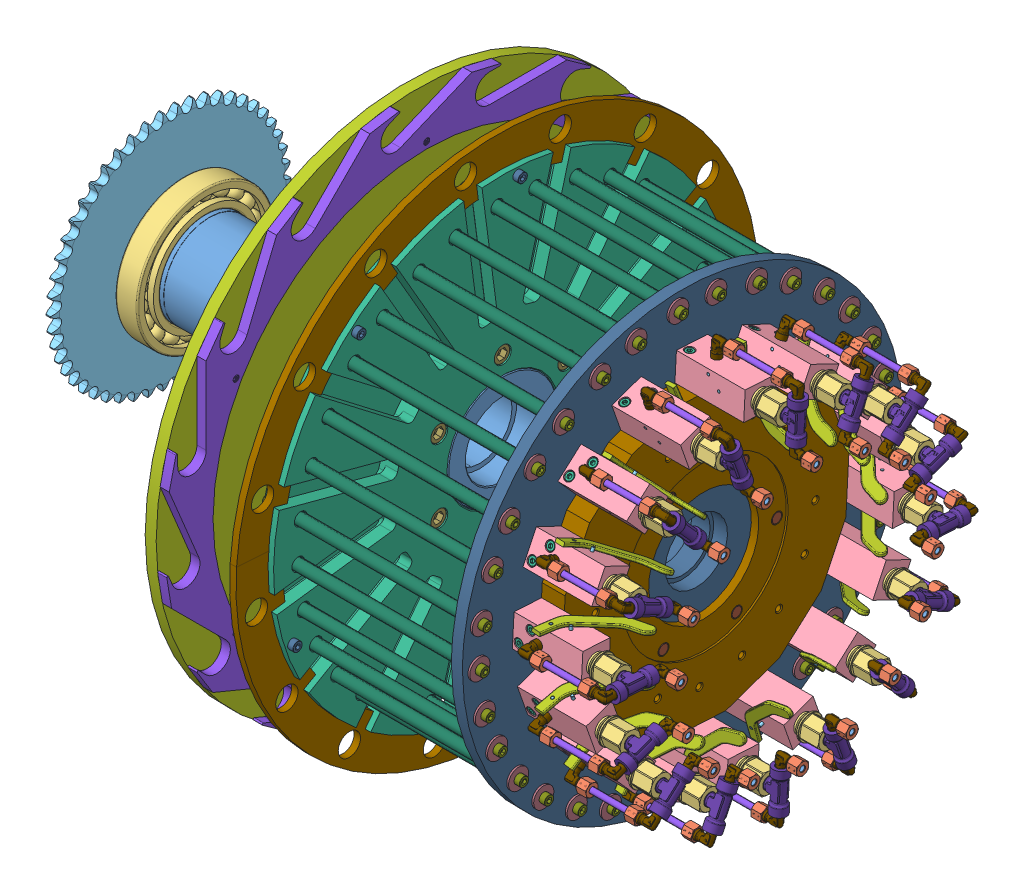
SolidWorks assembly assieme parte rotante, configuration Default. Lengths in mm.
Overall size (749.63 778.63 778.63).
555 component instances, 28 part files, 77 mates.
Components (placement in the parent):
- albero rotazione piatti-1: albero rotazione piatti [Default] at (60.413 18.3637 415) size (415 200 200)
- seger 100mm-1: seger 100mm [KS 1336 E - 100] at (-146.4567 18.3637 415) x (0 0 -1) z (1 0 0) size (107.55 112.98 3)
- SKF - 6020 - 20,DE,NC,20_68-1: SKF - 6020 - 20,DE,NC,20_68 [SKF - 6020 - 20,DE,NC,20_68] at (-131.4567 18.3637 415) x (1 0 0) z (0 -0.434476 -0.900684) size (24 150 150)
- calettatore d95-1: calettatore d95 [Default] at (-178.8867 18.3637 415) size (39.5 135 135)
- Chain wheel ISO - 50Z 10A-1-1: Chain wheel ISO - 50Z 10A-1 [Chain wheel ISO - 50Z 10A-1 --50SB120H25L95.0N] at (-164.8867 18.3637 415) size (33.93 262.06 262.51)
- Disco supporto montaggio e Colonne-1: Disco supporto montaggio e Colonne [Default] at (204.0433 18.3637 415) x (0 -0.866025 -0.5) z (1 0 0) size (499.6 499.6 29)
- SKF - 6020 - 20,DE,NC,20_68-2: SKF - 6020 - 20,DE,NC,20_68 [SKF - 6020 - 20,DE,NC,20_68] at (62.0433 18.3637 415) x (1 0 0) z (0 -0.432628 -0.901573) size (24 150 150)
- piatto rotante porta tappi-1: piatto rotante porta tappi [Default] at (99.0433 18.3637 415) x (0 0 -1) z (1 0 0) size (570 570 20.57)
- disco trasportatore tappi 31-1: disco trasportatore tappi 31 [Default] at (111.0433 18.3637 415) x (0 0.5 -0.866025) z (1 0 0) size (570 570 10.42)
- Distributore Rotante-1: Distributore Rotante [Default] at (425.0433 18.3637 415) x (0 -0.055301 -0.99847) z (1 0 0) size (310 310 25.54)
- disco trascinato porta distributore vuoto-1: disco trascinato porta distributore vuoto [Default] at (400.0433 18.3637 415) x (0 0.055301 0.99847) z (-1 0 0) size (480 480 50)
- m12 35mm-1: m12 35mm [ISO 4762 M12 x 35 - 35N] at (376.0433 -53.0243 378.8925) x (1 0 0) z (0 -0.5 0.866025) size (47 18 18)
- m12 90mm-3: m12 90mm [ISO 4762 M12 x 90 - 90N] at (203.0433 -21.6363 345.718) x (-1 0 0) z (0 -0.5 0.866025) size (102 18 18)
- rondella m6 22mm-1: rondella m6 22mm [Washer ISO 7094 - 6] at (99.0433 -101.6363 207.1539) x (1 0 0) z (0 -1 0) size (2 22 22)
- M6 20mm-1: M6 20mm [ISO 4762 M6 x 20 - 20N] at (91.0433 -101.6363 207.1539) x (1 0 0) z (0 0.5 0.866025) size (26 10 10)
- m12 35mm-2: m12 35mm [ISO 4762 M12 x 35 - 35N] at (376.0433 13.9397 335.1224) x (1 0 0) z (0 -1 0) size (47 18 18)
- m12 35mm-3: m12 35mm [ISO 4762 M12 x 35 - 35N] at (376.0433 85.3277 371.2299) x (1 0 0) z (0 -0.5 -0.866025) size (47 18 18)
- m12 35mm-4: m12 35mm [ISO 4762 M12 x 35 - 35N] at (376.0433 89.7517 451.1075) x (1 0 0) z (0 0.5 -0.866025) size (47 18 18)
- m12 35mm-5: m12 35mm [ISO 4762 M12 x 35 - 35N] at (376.0433 22.7877 494.8776) x (1 0 0) z (0 1 0) size (47 18 18)
- m12 35mm-6: m12 35mm [ISO 4762 M12 x 35 - 35N] at (376.0433 -48.6003 458.7701) x (1 0 0) z (0 0.5 0.866025) size (47 18 18)
- rondella m6 22mm-2: rondella m6 22mm [Washer ISO 7094 - 6] at (99.0433 138.3637 207.1539) x (1 0 0) z (0 -0.5 -0.866025) size (2 22 22)
- rondella m6 22mm-3: rondella m6 22mm [Washer ISO 7094 - 6] at (99.0433 258.3637 415) x (1 0 0) z (0 0.5 -0.866025) size (2 22 22)
- rondella m6 22mm-4: rondella m6 22mm [Washer ISO 7094 - 6] at (99.0433 138.3637 622.8461) x (1 0 0) z (0 1 0) size (2 22 22)
- rondella m6 22mm-5: rondella m6 22mm [Washer ISO 7094 - 6] at (99.0433 -101.6363 622.8461) x (1 0 0) z (0 0.5 0.866025) size (2 22 22)
- rondella m6 22mm-6: rondella m6 22mm [Washer ISO 7094 - 6] at (99.0433 -221.6363 415) x (1 0 0) z (0 -0.5 0.866025) size (2 22 22)
- M6 20mm-2: M6 20mm [ISO 4762 M6 x 20 - 20N] at (91.0433 138.3637 207.1539) x (1 0 0) z (0 -0.5 0.866025) size (26 10 10)
- M6 20mm-3: M6 20mm [ISO 4762 M6 x 20 - 20N] at (91.0433 258.3637 415) x (1 0 0) z (0 -1 0) size (26 10 10)
- M6 20mm-4: M6 20mm [ISO 4762 M6 x 20 - 20N] at (91.0433 138.3637 622.8461) x (1 0 0) z (0 -0.5 -0.866025) size (26 10 10)
- M6 20mm-5: M6 20mm [ISO 4762 M6 x 20 - 20N] at (91.0433 -101.6363 622.8461) x (1 0 0) z (0 0.5 -0.866025) size (26 10 10)
- M6 20mm-6: M6 20mm [ISO 4762 M6 x 20 - 20N] at (91.0433 -221.6363 415) x (1 0 0) z (0 1 0) size (26 10 10)
- m12 90mm-4: m12 90mm [ISO 4762 M12 x 90 - 90N] at (203.0433 58.3637 345.718) x (-1 0 0) z (0 -1 0) size (102 18 18)
- m12 90mm-5: m12 90mm [ISO 4762 M12 x 90 - 90N] at (203.0433 98.3637 415) x (-1 0 0) z (0 -0.5 -0.866025) size (102 18 18)
- m12 90mm-6: m12 90mm [ISO 4762 M12 x 90 - 90N] at (203.0433 58.3637 484.282) x (-1 0 0) z (0 0.5 -0.866025) size (102 18 18)
- m12 90mm-7: m12 90mm [ISO 4762 M12 x 90 - 90N] at (203.0433 -21.6363 484.282) x (-1 0 0) z (0 1 0) size (102 18 18)
- m12 90mm-8: m12 90mm [ISO 4762 M12 x 90 - 90N] at (203.0433 -61.6363 415) x (-1 0 0) z (0 0.5 0.866025) size (102 18 18)
- asta scorrimento carello-1: asta scorrimento carello [Default] at (287.5433 70.1437 197.9013) x (0 0 -1) z (1 0 0) size (12 12 225)
- rondella m6 22mm-7: rondella m6 22mm [Washer ISO 7094 - 6] at (175.0433 70.1437 197.9013) x (1 0 0) z (0 -1 0) size (2 22 22)
- M6 16mm-1: M6 16mm [ISO 4762 M6 x 16 - 16N] at (167.0433 70.1437 197.9013) size (22 10 10)
- M6 16mm-2: M6 16mm [ISO 4762 M6 x 16 - 16N] at (408.0433 70.1437 197.9013) x (-1 0 0) z (0 0 -1) size (22 10 10)
- rondella m6 22mm-8: rondella m6 22mm [Washer ISO 7094 - 6] at (400.0433 70.1437 197.9013) x (-1 0 0) z (0 1 0) size (2 22 22)
- rondella m6 22mm-9: rondella m6 22mm [Washer ISO 7094 - 6] at (175.0433 24.5373 191.8971) x (1 0 0) z (0 -0.965926 -0.258819) size (2 22 22)
- M6 16mm-3: M6 16mm [ISO 4762 M6 x 16 - 16N] at (167.0433 24.5373 191.8971) x (1 0 0) z (0 0.258819 -0.965926) size (22 10 10)
- asta scorrimento carello-2: asta scorrimento carello [Default] at (287.5433 24.5373 191.8971) x (0 0.258819 -0.965926) z (-1 0 0) size (12 12 225)
- rondella m6 22mm-10: rondella m6 22mm [Washer ISO 7094 - 6] at (400.0433 24.5373 191.8971) x (-1 0 0) z (0 0.965926 0.258819) size (2 22 22)
- M6 16mm-4: M6 16mm [ISO 4762 M6 x 16 - 16N] at (408.0433 24.5373 191.8971) x (-1 0 0) z (0 -0.258819 0.965926) size (22 10 10)
- AssiemeValvola-1: AssiemeValvola [Default] at (515.3257 74.6348 254.5832) x (0 -0.331007 0.943628) z (0 0.943628 0.331007) size (90.26 138.63 38)
  - RaccordoT-1: RaccordoT [Default] at origin size (43 29.75 16.5)
  - Raccordo a L-1: Raccordo a L [Default] at (-30 0 0) x (0 -1 0) z (0 0 -1) size (28.34 25.51 14.01)
    - 1809_06_10_01-1: 1809_06_10_01 [Default] at origin size (22.49 23 10)
    - 1809_06_10_02-1: 1809_06_10_02 [Default] at origin size (6.5 8.5 8.5)
    - 1809_06_10_03-1: 1809_06_10_03 [Default] at origin size (11.02 15.01 14.01)
  - Raccordo a L-2: Raccordo a L [Default] at (30 0 0) x (0 1 0) z (0 0 -1) size (28.34 25.51 14.01)
    - 1809_06_10_01-1: 1809_06_10_01 [Default] at origin size (22.49 23 10)
    - 1809_06_10_02-1: 1809_06_10_02 [Default] at origin size (6.5 8.5 8.5)
    - 1809_06_10_03-1: 1809_06_10_03 [Default] at origin size (11.02 15.01 14.01)
  - TappoChiusura-1: TappoChiusura [Default] at (0 -32 0) x (0 -1 0) z (0 0 1) size (38.28 26.74 26.74)
  - CorpoValvola-1: CorpoValvola [Default] at (-15 -115.2824 0) size (30 75 34)
  - Raccordo a L-3: Raccordo a L [Default] at (-30 -88.2824 0) x (0 1 0) z (0 0 1) size (28.34 25.51 14.01)
    - 1809_06_10_01-1: 1809_06_10_01 [Default] at origin size (22.49 23 10)
    - 1809_06_10_02-1: 1809_06_10_02 [Default] at origin size (6.5 8.5 8.5)
    - 1809_06_10_03-1: 1809_06_10_03 [Default] at origin size (11.02 15.01 14.01)
  - Spina_3x38-1: Spina_3x38 [Default] at (0 -68.2824 -21) x (-1 0 0) z (0 0 1) size (3 3 38)
  - Spina_3x38-2: Spina_3x38 [Default] at (-10 -80.2824 -21) x (0.996193 0.087174 0) z (0 0 1) size (3 3 38)
  - M5 40mm-3: M5 40mm [ISO 4762 M5 x 40 - 40N] at (-14.6 -108.7824 9) size (45 8.5 8.5)
  - M5 40mm-2: M5 40mm [ISO 4762 M5 x 40 - 40N] at (-14.6 -96.7824 -9) size (45 8.5 8.5)
  - LevaValvola-1: LevaValvola [Default] at (-24.507 -86.571 -17) x (0.996193 0.087174 0) z (0 0 1) size (77.55 60.2 4)
  - Tubo-1: Tubo [Default] at (-30 -15.9665 0) x (1 0 0) z (0 -1 0) size (6 6 56.4)
- M6 16mm-5: M6 16mm [ISO 4762 M6 x 16 - 16N] at (167.0433 -16.8778 194.6116) x (1 0 0) z (0 0.382683 0.92388) size (22 10 10)
- M6 16mm-6: M6 16mm [ISO 4762 M6 x 16 - 16N] at (167.0433 -98.5342 224.874) x (1 0 0) z (0 0.707107 0.707107) size (22 10 10)
- M6 16mm-7: M6 16mm [ISO 4762 M6 x 16 - 16N] at (167.0433 -162.3939 284.0814) x (1 0 0) z (0 0.92388 0.382683) size (22 10 10)
- M6 16mm-8: M6 16mm [ISO 4762 M6 x 16 - 16N] at (167.0433 -198.735 363.22) x (1 0 0) z (0 1 0) size (22 10 10)
- M6 16mm-9: M6 16mm [ISO 4762 M6 x 16 - 16N] at (167.0433 -202.0247 450.2415) x (1 0 0) z (0 0.92388 -0.382683) size (22 10 10)
- M6 16mm-10: M6 16mm [ISO 4762 M6 x 16 - 16N] at (167.0433 -171.7623 531.8979) x (1 0 0) z (0 0.707107 -0.707107) size (22 10 10)
- M6 16mm-11: M6 16mm [ISO 4762 M6 x 16 - 16N] at (167.0433 -112.5549 595.7576) x (1 0 0) z (0 0.382683 -0.92388) size (22 10 10)
- M6 16mm-12: M6 16mm [ISO 4762 M6 x 16 - 16N] at (167.0433 -33.4163 632.0987) x (1 0 0) z (0 0 -1) size (22 10 10)
- M6 16mm-13: M6 16mm [ISO 4762 M6 x 16 - 16N] at (167.0433 53.6052 635.3884) x (1 0 0) z (0 -0.382683 -0.92388) size (22 10 10)
- M6 16mm-14: M6 16mm [ISO 4762 M6 x 16 - 16N] at (167.0433 135.2616 605.126) x (1 0 0) z (0 -0.707107 -0.707107) size (22 10 10)
- M6 16mm-15: M6 16mm [ISO 4762 M6 x 16 - 16N] at (167.0433 199.1213 545.9186) x (1 0 0) z (0 -0.92388 -0.382683) size (22 10 10)
- M6 16mm-16: M6 16mm [ISO 4762 M6 x 16 - 16N] at (167.0433 235.4624 466.78) x (1 0 0) z (0 -1 0) size (22 10 10)
- M6 16mm-17: M6 16mm [ISO 4762 M6 x 16 - 16N] at (167.0433 238.7521 379.7585) x (1 0 0) z (0 -0.92388 0.382683) size (22 10 10)
- M6 16mm-18: M6 16mm [ISO 4762 M6 x 16 - 16N] at (167.0433 208.4897 298.1021) x (1 0 0) z (0 -0.707107 0.707107) size (22 10 10)
- M6 16mm-19: M6 16mm [ISO 4762 M6 x 16 - 16N] at (167.0433 149.2823 234.2424) x (1 0 0) z (0 -0.382683 0.92388) size (22 10 10)
- rondella m6 22mm-11: rondella m6 22mm [Washer ISO 7094 - 6] at (175.0433 -16.8778 194.6116) x (1 0 0) z (0 -0.92388 0.382683) size (2 22 22)
- rondella m6 22mm-12: rondella m6 22mm [Washer ISO 7094 - 6] at (175.0433 -98.5342 224.874) x (1 0 0) z (0 -0.707107 0.707107) size (2 22 22)
- rondella m6 22mm-13: rondella m6 22mm [Washer ISO 7094 - 6] at (175.0433 -162.3939 284.0814) x (1 0 0) z (0 -0.382683 0.92388) size (2 22 22)
- rondella m6 22mm-14: rondella m6 22mm [Washer ISO 7094 - 6] at (175.0433 -198.735 363.22) size (2 22 22)
- rondella m6 22mm-15: rondella m6 22mm [Washer ISO 7094 - 6] at (175.0433 -202.0247 450.2415) x (1 0 0) z (0 0.382683 0.92388) size (2 22 22)
- rondella m6 22mm-16: rondella m6 22mm [Washer ISO 7094 - 6] at (175.0433 -171.7623 531.8979) x (1 0 0) z (0 0.707107 0.707107) size (2 22 22)
- rondella m6 22mm-17: rondella m6 22mm [Washer ISO 7094 - 6] at (175.0433 -112.5549 595.7576) x (1 0 0) z (0 0.92388 0.382683) size (2 22 22)
- rondella m6 22mm-18: rondella m6 22mm [Washer ISO 7094 - 6] at (175.0433 -33.4163 632.0987) x (1 0 0) z (0 1 0) size (2 22 22)
- rondella m6 22mm-19: rondella m6 22mm [Washer ISO 7094 - 6] at (175.0433 53.6052 635.3884) x (1 0 0) z (0 0.92388 -0.382683) size (2 22 22)
- rondella m6 22mm-20: rondella m6 22mm [Washer ISO 7094 - 6] at (175.0433 135.2616 605.126) x (1 0 0) z (0 0.707107 -0.707107) size (2 22 22)
- rondella m6 22mm-21: rondella m6 22mm [Washer ISO 7094 - 6] at (175.0433 199.1213 545.9186) x (1 0 0) z (0 0.382683 -0.92388) size (2 22 22)
- rondella m6 22mm-22: rondella m6 22mm [Washer ISO 7094 - 6] at (175.0433 235.4624 466.78) x (1 0 0) z (0 0 -1) size (2 22 22)
- rondella m6 22mm-23: rondella m6 22mm [Washer ISO 7094 - 6] at (175.0433 238.7521 379.7585) x (1 0 0) z (0 -0.382683 -0.92388) size (2 22 22)
- rondella m6 22mm-24: rondella m6 22mm [Washer ISO 7094 - 6] at (175.0433 208.4897 298.1021) x (1 0 0) z (0 -0.707107 -0.707107) size (2 22 22)
- rondella m6 22mm-25: rondella m6 22mm [Washer ISO 7094 - 6] at (175.0433 149.2823 234.2424) x (1 0 0) z (0 -0.92388 -0.382683) size (2 22 22)
- asta scorrimento carello-3: asta scorrimento carello [Default] at (287.5433 -16.8778 194.6116) x (0 -0.382683 -0.92388) z (1 0 0) size (12 12 225)
- asta scorrimento carello-4: asta scorrimento carello [Default] at (287.5433 -98.5342 224.874) x (0 -0.707107 -0.707107) z (1 0 0) size (12 12 225)
- asta scorrimento carello-5: asta scorrimento carello [Default] at (287.5433 -162.3939 284.0814) x (0 -0.92388 -0.382683) z (1 0 0) size (12 12 225)
- asta scorrimento carello-6: asta scorrimento carello [Default] at (287.5433 -198.735 363.22) x (0 -1 0) z (1 0 0) size (12 12 225)
- asta scorrimento carello-7: asta scorrimento carello [Default] at (287.5433 -202.0247 450.2415) x (0 -0.92388 0.382683) z (1 0 0) size (12 12 225)
- asta scorrimento carello-8: asta scorrimento carello [Default] at (287.5433 -171.7623 531.8979) x (0 -0.707107 0.707107) z (1 0 0) size (12 12 225)
- asta scorrimento carello-9: asta scorrimento carello [Default] at (287.5433 -112.5549 595.7576) x (0 -0.382683 0.92388) z (1 0 0) size (12 12 225)
- asta scorrimento carello-10: asta scorrimento carello [Default] at (287.5433 -33.4163 632.0987) x (0 0 1) z (1 0 0) size (12 12 225)
- asta scorrimento carello-11: asta scorrimento carello [Default] at (287.5433 53.6052 635.3884) x (0 0.382683 0.92388) z (1 0 0) size (12 12 225)
- asta scorrimento carello-12: asta scorrimento carello [Default] at (287.5433 135.2616 605.126) x (0 0.707107 0.707107) z (1 0 0) size (12 12 225)
- asta scorrimento carello-13: asta scorrimento carello [Default] at (287.5433 199.1213 545.9186) x (0 0.92388 0.382683) z (1 0 0) size (12 12 225)
- asta scorrimento carello-14: asta scorrimento carello [Default] at (287.5433 235.4624 466.78) x (0 1 0) z (1 0 0) size (12 12 225)
- asta scorrimento carello-15: asta scorrimento carello [Default] at (287.5433 238.7521 379.7585) x (0 0.92388 -0.382683) z (1 0 0) size (12 12 225)
- asta scorrimento carello-16: asta scorrimento carello [Default] at (287.5433 208.4897 298.1021) x (0 0.707107 -0.707107) z (1 0 0) size (12 12 225)
- asta scorrimento carello-17: asta scorrimento carello [Default] at (287.5433 149.2823 234.2424) x (0 0.382683 -0.92388) z (1 0 0) size (12 12 225)
- M6 16mm-20: M6 16mm [ISO 4762 M6 x 16 - 16N] at (408.0433 -16.8778 194.6116) x (-1 0 0) z (0 -0.382683 -0.92388) size (22 10 10)
- M6 16mm-21: M6 16mm [ISO 4762 M6 x 16 - 16N] at (408.0433 -98.5342 224.874) x (-1 0 0) z (0 -0.707107 -0.707107) size (22 10 10)
- M6 16mm-22: M6 16mm [ISO 4762 M6 x 16 - 16N] at (408.0433 -162.3939 284.0814) x (-1 0 0) z (0 -0.92388 -0.382683) size (22 10 10)
- M6 16mm-23: M6 16mm [ISO 4762 M6 x 16 - 16N] at (408.0433 -198.735 363.22) x (-1 0 0) z (0 -1 0) size (22 10 10)
- M6 16mm-24: M6 16mm [ISO 4762 M6 x 16 - 16N] at (408.0433 -202.0247 450.2415) x (-1 0 0) z (0 -0.92388 0.382683) size (22 10 10)
- M6 16mm-25: M6 16mm [ISO 4762 M6 x 16 - 16N] at (408.0433 -171.7623 531.8979) x (-1 0 0) z (0 -0.707107 0.707107) size (22 10 10)
- M6 16mm-26: M6 16mm [ISO 4762 M6 x 16 - 16N] at (408.0433 -112.5549 595.7576) x (-1 0 0) z (0 -0.382683 0.92388) size (22 10 10)
- M6 16mm-27: M6 16mm [ISO 4762 M6 x 16 - 16N] at (408.0433 -33.4163 632.0987) x (-1 0 0) z (0 0 1) size (22 10 10)
- M6 16mm-28: M6 16mm [ISO 4762 M6 x 16 - 16N] at (408.0433 53.6052 635.3884) x (-1 0 0) z (0 0.382683 0.92388) size (22 10 10)
- M6 16mm-29: M6 16mm [ISO 4762 M6 x 16 - 16N] at (408.0433 135.2616 605.126) x (-1 0 0) z (0 0.707107 0.707107) size (22 10 10)
- M6 16mm-30: M6 16mm [ISO 4762 M6 x 16 - 16N] at (408.0433 199.1213 545.9186) x (-1 0 0) z (0 0.92388 0.382683) size (22 10 10)
- M6 16mm-31: M6 16mm [ISO 4762 M6 x 16 - 16N] at (408.0433 235.4624 466.78) x (-1 0 0) z (0 1 0) size (22 10 10)
- M6 16mm-32: M6 16mm [ISO 4762 M6 x 16 - 16N] at (408.0433 238.7521 379.7585) x (-1 0 0) z (0 0.92388 -0.382683) size (22 10 10)
- M6 16mm-33: M6 16mm [ISO 4762 M6 x 16 - 16N] at (408.0433 208.4897 298.1021) x (-1 0 0) z (0 0.707107 -0.707107) size (22 10 10)
- M6 16mm-34: M6 16mm [ISO 4762 M6 x 16 - 16N] at (408.0433 149.2823 234.2424) x (-1 0 0) z (0 0.382683 -0.92388) size (22 10 10)
- rondella m6 22mm-26: rondella m6 22mm [Washer ISO 7094 - 6] at (400.0433 -16.8778 194.6116) x (-1 0 0) z (0 0.92388 -0.382683) size (2 22 22)
- rondella m6 22mm-27: rondella m6 22mm [Washer ISO 7094 - 6] at (400.0433 -98.5342 224.874) x (-1 0 0) z (0 0.707107 -0.707107) size (2 22 22)
- rondella m6 22mm-28: rondella m6 22mm [Washer ISO 7094 - 6] at (400.0433 -162.3939 284.0814) x (-1 0 0) z (0 0.382683 -0.92388) size (2 22 22)
- rondella m6 22mm-29: rondella m6 22mm [Washer ISO 7094 - 6] at (400.0433 -198.735 363.22) x (-1 0 0) z (0 0 -1) size (2 22 22)
- rondella m6 22mm-30: rondella m6 22mm [Washer ISO 7094 - 6] at (400.0433 -202.0247 450.2415) x (-1 0 0) z (0 -0.382683 -0.92388) size (2 22 22)
- rondella m6 22mm-31: rondella m6 22mm [Washer ISO 7094 - 6] at (400.0433 -171.7623 531.8979) x (-1 0 0) z (0 -0.707107 -0.707107) size (2 22 22)
- rondella m6 22mm-32: rondella m6 22mm [Washer ISO 7094 - 6] at (400.0433 -112.5549 595.7576) x (-1 0 0) z (0 -0.92388 -0.382683) size (2 22 22)
- rondella m6 22mm-33: rondella m6 22mm [Washer ISO 7094 - 6] at (400.0433 -33.4163 632.0987) x (-1 0 0) z (0 -1 0) size (2 22 22)
- rondella m6 22mm-34: rondella m6 22mm [Washer ISO 7094 - 6] at (400.0433 53.6052 635.3884) x (-1 0 0) z (0 -0.92388 0.382683) size (2 22 22)
- rondella m6 22mm-35: rondella m6 22mm [Washer ISO 7094 - 6] at (400.0433 135.2616 605.126) x (-1 0 0) z (0 -0.707107 0.707107) size (2 22 22)
- rondella m6 22mm-36: rondella m6 22mm [Washer ISO 7094 - 6] at (400.0433 199.1213 545.9186) x (-1 0 0) z (0 -0.382683 0.92388) size (2 22 22)
- rondella m6 22mm-37: rondella m6 22mm [Washer ISO 7094 - 6] at (400.0433 235.4624 466.78) x (-1 0 0) z (0 0 1) size (2 22 22)
- rondella m6 22mm-38: rondella m6 22mm [Washer ISO 7094 - 6] at (400.0433 238.7521 379.7585) x (-1 0 0) z (0 0.382683 0.92388) size (2 22 22)
- rondella m6 22mm-39: rondella m6 22mm [Washer ISO 7094 - 6] at (400.0433 208.4897 298.1021) x (-1 0 0) z (0 0.707107 0.707107) size (2 22 22)
- rondella m6 22mm-40: rondella m6 22mm [Washer ISO 7094 - 6] at (400.0433 149.2823 234.2424) x (-1 0 0) z (0 0.92388 0.382683) size (2 22 22)
- rondella m6 22mm-41: rondella m6 22mm [Washer ISO 7094 - 6] at (175.0433 -61.3104 206.5173) x (1 0 0) z (0 -0.991445 0.130526) size (2 22 22)
- rondella m6 22mm-42: rondella m6 22mm [Washer ISO 7094 - 6] at (175.0433 -135.0285 252.8771) x (1 0 0) z (0 -0.866025 0.5) size (2 22 22)
- rondella m6 22mm-43: rondella m6 22mm [Washer ISO 7094 - 6] at (175.0433 -185.3939 323.9186) x (1 0 0) z (0 -0.608761 0.793353) size (2 22 22)
- rondella m6 22mm-44: rondella m6 22mm [Washer ISO 7094 - 6] at (175.0433 -204.7392 408.8264) x (1 0 0) z (0 -0.258819 0.965926) size (2 22 22)
- rondella m6 22mm-45: rondella m6 22mm [Washer ISO 7094 - 6] at (175.0433 -190.119 494.6741) x (1 0 0) z (0 0.130526 0.991445) size (2 22 22)
- rondella m6 22mm-46: rondella m6 22mm [Washer ISO 7094 - 6] at (175.0433 -143.7592 568.3922) x (1 0 0) z (0 0.5 0.866025) size (2 22 22)
- rondella m6 22mm-47: rondella m6 22mm [Washer ISO 7094 - 6] at (175.0433 -72.7177 618.7576) x (1 0 0) z (0 0.793353 0.608761) size (2 22 22)
- rondella m6 22mm-48: rondella m6 22mm [Washer ISO 7094 - 6] at (175.0433 12.1901 638.1029) x (1 0 0) z (0 0.965926 0.258819) size (2 22 22)
- rondella m6 22mm-49: rondella m6 22mm [Washer ISO 7094 - 6] at (175.0433 98.0378 623.4827) x (1 0 0) z (0 0.991445 -0.130526) size (2 22 22)
- rondella m6 22mm-50: rondella m6 22mm [Washer ISO 7094 - 6] at (175.0433 171.7559 577.1229) x (1 0 0) z (0 0.866025 -0.5) size (2 22 22)
- rondella m6 22mm-51: rondella m6 22mm [Washer ISO 7094 - 6] at (175.0433 222.1213 506.0814) x (1 0 0) z (0 0.608761 -0.793353) size (2 22 22)
- rondella m6 22mm-52: rondella m6 22mm [Washer ISO 7094 - 6] at (175.0433 241.4666 421.1736) x (1 0 0) z (0 0.258819 -0.965926) size (2 22 22)
- rondella m6 22mm-53: rondella m6 22mm [Washer ISO 7094 - 6] at (175.0433 226.8464 335.3259) x (1 0 0) z (0 -0.130526 -0.991445) size (2 22 22)
- rondella m6 22mm-54: rondella m6 22mm [Washer ISO 7094 - 6] at (175.0433 180.4866 261.6078) x (1 0 0) z (0 -0.5 -0.866025) size (2 22 22)
- rondella m6 22mm-55: rondella m6 22mm [Washer ISO 7094 - 6] at (175.0433 109.4451 211.2424) x (1 0 0) z (0 -0.793353 -0.608761) size (2 22 22)
- M6 16mm-35: M6 16mm [ISO 4762 M6 x 16 - 16N] at (167.0433 -61.3104 206.5173) x (1 0 0) z (0 -0.130526 -0.991445) size (22 10 10)
- M6 16mm-36: M6 16mm [ISO 4762 M6 x 16 - 16N] at (167.0433 -135.0285 252.8771) x (1 0 0) z (0 -0.5 -0.866025) size (22 10 10)
- M6 16mm-37: M6 16mm [ISO 4762 M6 x 16 - 16N] at (167.0433 -185.3939 323.9186) x (1 0 0) z (0 -0.793353 -0.608761) size (22 10 10)
- M6 16mm-38: M6 16mm [ISO 4762 M6 x 16 - 16N] at (167.0433 -204.7392 408.8264) x (1 0 0) z (0 -0.965926 -0.258819) size (22 10 10)
- M6 16mm-39: M6 16mm [ISO 4762 M6 x 16 - 16N] at (167.0433 -190.119 494.6741) x (1 0 0) z (0 -0.991445 0.130526) size (22 10 10)
- M6 16mm-40: M6 16mm [ISO 4762 M6 x 16 - 16N] at (167.0433 -143.7592 568.3922) x (1 0 0) z (0 -0.866025 0.5) size (22 10 10)
- M6 16mm-41: M6 16mm [ISO 4762 M6 x 16 - 16N] at (167.0433 -72.7177 618.7576) x (1 0 0) z (0 -0.608761 0.793353) size (22 10 10)
- M6 16mm-42: M6 16mm [ISO 4762 M6 x 16 - 16N] at (167.0433 12.1901 638.1029) x (1 0 0) z (0 -0.258819 0.965926) size (22 10 10)
- M6 16mm-43: M6 16mm [ISO 4762 M6 x 16 - 16N] at (167.0433 98.0378 623.4827) x (1 0 0) z (0 0.130526 0.991445) size (22 10 10)
- M6 16mm-44: M6 16mm [ISO 4762 M6 x 16 - 16N] at (167.0433 171.7559 577.1229) x (1 0 0) z (0 0.5 0.866025) size (22 10 10)
- M6 16mm-45: M6 16mm [ISO 4762 M6 x 16 - 16N] at (167.0433 222.1213 506.0814) x (1 0 0) z (0 0.793353 0.608761) size (22 10 10)
- M6 16mm-46: M6 16mm [ISO 4762 M6 x 16 - 16N] at (167.0433 241.4666 421.1736) x (1 0 0) z (0 0.965926 0.258819) size (22 10 10)
- M6 16mm-47: M6 16mm [ISO 4762 M6 x 16 - 16N] at (167.0433 226.8464 335.3259) x (1 0 0) z (0 0.991445 -0.130526) size (22 10 10)
- M6 16mm-48: M6 16mm [ISO 4762 M6 x 16 - 16N] at (167.0433 180.4866 261.6078) x (1 0 0) z (0 0.866025 -0.5) size (22 10 10)
- M6 16mm-49: M6 16mm [ISO 4762 M6 x 16 - 16N] at (167.0433 109.4451 211.2424) x (1 0 0) z (0 0.608761 -0.793353) size (22 10 10)
- asta scorrimento carello-18: asta scorrimento carello [Default] at (287.5433 -61.3104 206.5173) x (0 -0.130526 -0.991445) z (-1 0 0) size (12 12 225)
- asta scorrimento carello-19: asta scorrimento carello [Default] at (287.5433 -135.0285 252.8771) x (0 -0.5 -0.866025) z (-1 0 0) size (12 12 225)
- asta scorrimento carello-20: asta scorrimento carello [Default] at (287.5433 -185.3939 323.9186) x (0 -0.793353 -0.608761) z (-1 0 0) size (12 12 225)
- asta scorrimento carello-21: asta scorrimento carello [Default] at (287.5433 -204.7392 408.8264) x (0 -0.965926 -0.258819) z (-1 0 0) size (12 12 225)
- asta scorrimento carello-22: asta scorrimento carello [Default] at (287.5433 -190.119 494.6741) x (0 -0.991445 0.130526) z (-1 0 0) size (12 12 225)
- asta scorrimento carello-23: asta scorrimento carello [Default] at (287.5433 -143.7592 568.3922) x (0 -0.866025 0.5) z (-1 0 0) size (12 12 225)
- asta scorrimento carello-24: asta scorrimento carello [Default] at (287.5433 -72.7177 618.7576) x (0 -0.608761 0.793353) z (-1 0 0) size (12 12 225)
- asta scorrimento carello-25: asta scorrimento carello [Default] at (287.5433 12.1901 638.1029) x (0 -0.258819 0.965926) z (-1 0 0) size (12 12 225)
- asta scorrimento carello-26: asta scorrimento carello [Default] at (287.5433 98.0378 623.4827) x (0 0.130526 0.991445) z (-1 0 0) size (12 12 225)
- asta scorrimento carello-27: asta scorrimento carello [Default] at (287.5433 171.7559 577.1229) x (0 0.5 0.866025) z (-1 0 0) size (12 12 225)
- asta scorrimento carello-28: asta scorrimento carello [Default] at (287.5433 222.1213 506.0814) x (0 0.793353 0.608761) z (-1 0 0) size (12 12 225)
- asta scorrimento carello-29: asta scorrimento carello [Default] at (287.5433 241.4666 421.1736) x (0 0.965926 0.258819) z (-1 0 0) size (12 12 225)
- asta scorrimento carello-30: asta scorrimento carello [Default] at (287.5433 226.8464 335.3259) x (0 0.991445 -0.130526) z (-1 0 0) size (12 12 225)
- asta scorrimento carello-31: asta scorrimento carello [Default] at (287.5433 180.4866 261.6078) x (0 0.866025 -0.5) z (-1 0 0) size (12 12 225)
- asta scorrimento carello-32: asta scorrimento carello [Default] at (287.5433 109.4451 211.2424) x (0 0.608761 -0.793353) z (-1 0 0) size (12 12 225)
- rondella m6 22mm-56: rondella m6 22mm [Washer ISO 7094 - 6] at (400.0433 -61.3104 206.5173) x (-1 0 0) z (0 0.991445 -0.130526) size (2 22 22)
- rondella m6 22mm-57: rondella m6 22mm [Washer ISO 7094 - 6] at (400.0433 -135.0285 252.8771) x (-1 0 0) z (0 0.866025 -0.5) size (2 22 22)
- rondella m6 22mm-58: rondella m6 22mm [Washer ISO 7094 - 6] at (400.0433 -185.3939 323.9186) x (-1 0 0) z (0 0.608761 -0.793353) size (2 22 22)
- rondella m6 22mm-59: rondella m6 22mm [Washer ISO 7094 - 6] at (400.0433 -204.7392 408.8264) x (-1 0 0) z (0 0.258819 -0.965926) size (2 22 22)
- rondella m6 22mm-60: rondella m6 22mm [Washer ISO 7094 - 6] at (400.0433 -190.119 494.6741) x (-1 0 0) z (0 -0.130526 -0.991445) size (2 22 22)
- rondella m6 22mm-61: rondella m6 22mm [Washer ISO 7094 - 6] at (400.0433 -143.7592 568.3922) x (-1 0 0) z (0 -0.5 -0.866025) size (2 22 22)
- rondella m6 22mm-62: rondella m6 22mm [Washer ISO 7094 - 6] at (400.0433 -72.7177 618.7576) x (-1 0 0) z (0 -0.793353 -0.608761) size (2 22 22)
- rondella m6 22mm-63: rondella m6 22mm [Washer ISO 7094 - 6] at (400.0433 12.1901 638.1029) x (-1 0 0) z (0 -0.965926 -0.258819) size (2 22 22)
- rondella m6 22mm-64: rondella m6 22mm [Washer ISO 7094 - 6] at (400.0433 98.0378 623.4827) x (-1 0 0) z (0 -0.991445 0.130526) size (2 22 22)
- rondella m6 22mm-65: rondella m6 22mm [Washer ISO 7094 - 6] at (400.0433 171.7559 577.1229) x (-1 0 0) z (0 -0.866025 0.5) size (2 22 22)
- rondella m6 22mm-66: rondella m6 22mm [Washer ISO 7094 - 6] at (400.0433 222.1213 506.0814) x (-1 0 0) z (0 -0.608761 0.793353) size (2 22 22)
- rondella m6 22mm-67: rondella m6 22mm [Washer ISO 7094 - 6] at (400.0433 241.4666 421.1736) x (-1 0 0) z (0 -0.258819 0.965926) size (2 22 22)
- rondella m6 22mm-68: rondella m6 22mm [Washer ISO 7094 - 6] at (400.0433 226.8464 335.3259) x (-1 0 0) z (0 0.130526 0.991445) size (2 22 22)
- rondella m6 22mm-69: rondella m6 22mm [Washer ISO 7094 - 6] at (400.0433 180.4866 261.6078) x (-1 0 0) z (0 0.5 0.866025) size (2 22 22)
- rondella m6 22mm-70: rondella m6 22mm [Washer ISO 7094 - 6] at (400.0433 109.4451 211.2424) x (-1 0 0) z (0 0.793353 0.608761) size (2 22 22)
- M6 16mm-50: M6 16mm [ISO 4762 M6 x 16 - 16N] at (408.0433 -61.3104 206.5173) x (-1 0 0) z (0 0.130526 0.991445) size (22 10 10)
- M6 16mm-51: M6 16mm [ISO 4762 M6 x 16 - 16N] at (408.0433 -135.0285 252.8771) x (-1 0 0) z (0 0.5 0.866025) size (22 10 10)
- M6 16mm-52: M6 16mm [ISO 4762 M6 x 16 - 16N] at (408.0433 -185.3939 323.9186) x (-1 0 0) z (0 0.793353 0.608761) size (22 10 10)
- M6 16mm-53: M6 16mm [ISO 4762 M6 x 16 - 16N] at (408.0433 -204.7392 408.8264) x (-1 0 0) z (0 0.965926 0.258819) size (22 10 10)
- M6 16mm-54: M6 16mm [ISO 4762 M6 x 16 - 16N] at (408.0433 -190.119 494.6741) x (-1 0 0) z (0 0.991445 -0.130526) size (22 10 10)
- M6 16mm-55: M6 16mm [ISO 4762 M6 x 16 - 16N] at (408.0433 -143.7592 568.3922) x (-1 0 0) z (0 0.866025 -0.5) size (22 10 10)
- M6 16mm-56: M6 16mm [ISO 4762 M6 x 16 - 16N] at (408.0433 -72.7177 618.7576) x (-1 0 0) z (0 0.608761 -0.793353) size (22 10 10)
- M6 16mm-57: M6 16mm [ISO 4762 M6 x 16 - 16N] at (408.0433 12.1901 638.1029) x (-1 0 0) z (0 0.258819 -0.965926) size (22 10 10)
- M6 16mm-58: M6 16mm [ISO 4762 M6 x 16 - 16N] at (408.0433 98.0378 623.4827) x (-1 0 0) z (0 -0.130526 -0.991445) size (22 10 10)
- M6 16mm-59: M6 16mm [ISO 4762 M6 x 16 - 16N] at (408.0433 171.7559 577.1229) x (-1 0 0) z (0 -0.5 -0.866025) size (22 10 10)
- M6 16mm-60: M6 16mm [ISO 4762 M6 x 16 - 16N] at (408.0433 222.1213 506.0814) x (-1 0 0) z (0 -0.793353 -0.608761) size (22 10 10)
- M6 16mm-61: M6 16mm [ISO 4762 M6 x 16 - 16N] at (408.0433 241.4666 421.1736) x (-1 0 0) z (0 -0.965926 -0.258819) size (22 10 10)
- M6 16mm-62: M6 16mm [ISO 4762 M6 x 16 - 16N] at (408.0433 226.8464 335.3259) x (-1 0 0) z (0 -0.991445 0.130526) size (22 10 10)
- M6 16mm-63: M6 16mm [ISO 4762 M6 x 16 - 16N] at (408.0433 180.4866 261.6078) x (-1 0 0) z (0 -0.866025 0.5) size (22 10 10)
- M6 16mm-64: M6 16mm [ISO 4762 M6 x 16 - 16N] at (408.0433 109.4451 211.2424) x (-1 0 0) z (0 -0.608761 0.793353) size (22 10 10)
- AssiemeValvola-2: AssiemeValvola [Default] at (515.3257 8.9626 245.2601) x (0 0.055301 0.99847) z (0 0.99847 -0.055301) size (90.26 138.63 38)
  - RaccordoT-1: RaccordoT [Default] at origin size (43 29.75 16.5)
  - Raccordo a L-1: Raccordo a L [Default] at (-30 0 0) x (0 -1 0) z (0 0 -1) size (28.34 25.51 14.01)
    - 1809_06_10_01-1: 1809_06_10_01 [Default] at origin size (22.49 23 10)
    - 1809_06_10_02-1: 1809_06_10_02 [Default] at origin size (6.5 8.5 8.5)
    - 1809_06_10_03-1: 1809_06_10_03 [Default] at origin size (11.02 15.01 14.01)
  - Raccordo a L-2: Raccordo a L [Default] at (30 0 0) x (0 1 0) z (0 0 -1) size (28.34 25.51 14.01)
    - 1809_06_10_01-1: 1809_06_10_01 [Default] at origin size (22.49 23 10)
    - 1809_06_10_02-1: 1809_06_10_02 [Default] at origin size (6.5 8.5 8.5)
    - 1809_06_10_03-1: 1809_06_10_03 [Default] at origin size (11.02 15.01 14.01)
  - TappoChiusura-1: TappoChiusura [Default] at (0 -32 0) x (0 -1 0) z (0 0 1) size (38.28 26.74 26.74)
  - CorpoValvola-1: CorpoValvola [Default] at (-15 -115.2824 0) size (30 75 34)
  - Raccordo a L-3: Raccordo a L [Default] at (-30 -88.2824 0) x (0 1 0) z (0 0 1) size (28.34 25.51 14.01)
    - 1809_06_10_01-1: 1809_06_10_01 [Default] at origin size (22.49 23 10)
    - 1809_06_10_02-1: 1809_06_10_02 [Default] at origin size (6.5 8.5 8.5)
    - 1809_06_10_03-1: 1809_06_10_03 [Default] at origin size (11.02 15.01 14.01)
  - Spina_3x38-1: Spina_3x38 [Default] at (0 -68.2824 -21) x (-1 0 0) z (0 0 1) size (3 3 38)
  - Spina_3x38-2: Spina_3x38 [Default] at (-10 -80.2824 -21) x (0.996193 0.087174 0) z (0 0 1) size (3 3 38)
  - M5 40mm-3: M5 40mm [ISO 4762 M5 x 40 - 40N] at (-14.6 -108.7824 9) size (45 8.5 8.5)
  - M5 40mm-2: M5 40mm [ISO 4762 M5 x 40 - 40N] at (-14.6 -96.7824 -9) size (45 8.5 8.5)
  - LevaValvola-1: LevaValvola [Default] at (-24.507 -86.571 -17) x (0.996193 0.087174 0) z (0 0 1) size (77.55 60.2 4)
  - Tubo-1: Tubo [Default] at (-30 -15.9665 0) x (1 0 0) z (0 -1 0) size (6 6 56.4)
- AssiemeValvola-3: AssiemeValvola [Default] at (515.3257 -55.2784 261.7785) x (0 0.433189 0.901303) z (0 0.901303 -0.433189) size (90.26 138.63 38)
  - RaccordoT-1: RaccordoT [Default] at origin size (43 29.75 16.5)
  - Raccordo a L-1: Raccordo a L [Default] at (-30 0 0) x (0 -1 0) z (0 0 -1) size (28.34 25.51 14.01)
    - 1809_06_10_01-1: 1809_06_10_01 [Default] at origin size (22.49 23 10)
    - 1809_06_10_02-1: 1809_06_10_02 [Default] at origin size (6.5 8.5 8.5)
    - 1809_06_10_03-1: 1809_06_10_03 [Default] at origin size (11.02 15.01 14.01)
  - Raccordo a L-2: Raccordo a L [Default] at (30 0 0) x (0 1 0) z (0 0 -1) size (28.34 25.51 14.01)
    - 1809_06_10_01-1: 1809_06_10_01 [Default] at origin size (22.49 23 10)
    - 1809_06_10_02-1: 1809_06_10_02 [Default] at origin size (6.5 8.5 8.5)
    - 1809_06_10_03-1: 1809_06_10_03 [Default] at origin size (11.02 15.01 14.01)
  - TappoChiusura-1: TappoChiusura [Default] at (0 -32 0) x (0 -1 0) z (0 0 1) size (38.28 26.74 26.74)
  - CorpoValvola-1: CorpoValvola [Default] at (-15 -115.2824 0) size (30 75 34)
  - Raccordo a L-3: Raccordo a L [Default] at (-30 -88.2824 0) x (0 1 0) z (0 0 1) size (28.34 25.51 14.01)
    - 1809_06_10_01-1: 1809_06_10_01 [Default] at origin size (22.49 23 10)
    - 1809_06_10_02-1: 1809_06_10_02 [Default] at origin size (6.5 8.5 8.5)
    - 1809_06_10_03-1: 1809_06_10_03 [Default] at origin size (11.02 15.01 14.01)
  - Spina_3x38-1: Spina_3x38 [Default] at (0 -68.2824 -21) x (-1 0 0) z (0 0 1) size (3 3 38)
  - Spina_3x38-2: Spina_3x38 [Default] at (-10 -80.2824 -21) x (0.996193 0.087174 0) z (0 0 1) size (3 3 38)
  - M5 40mm-3: M5 40mm [ISO 4762 M5 x 40 - 40N] at (-14.6 -108.7824 9) size (45 8.5 8.5)
  - M5 40mm-2: M5 40mm [ISO 4762 M5 x 40 - 40N] at (-14.6 -96.7824 -9) size (45 8.5 8.5)
  - LevaValvola-1: LevaValvola [Default] at (-24.507 -86.571 -17) x (0.996193 0.087174 0) z (0 0 1) size (77.55 60.2 4)
  - Tubo-1: Tubo [Default] at (-30 -15.9665 0) x (1 0 0) z (0 -1 0) size (6 6 56.4)
- AssiemeValvola-4: AssiemeValvola [Default] at (515.3257 -108.3081 301.6234) x (0 0.745128 0.666921) z (0 0.666921 -0.745128) size (90.26 138.63 38)
  - RaccordoT-1: RaccordoT [Default] at origin size (43 29.75 16.5)
  - Raccordo a L-1: Raccordo a L [Default] at (-30 0 0) x (0 -1 0) z (0 0 -1) size (28.34 25.51 14.01)
    - 1809_06_10_01-1: 1809_06_10_01 [Default] at origin size (22.49 23 10)
    - 1809_06_10_02-1: 1809_06_10_02 [Default] at origin size (6.5 8.5 8.5)
    - 1809_06_10_03-1: 1809_06_10_03 [Default] at origin size (11.02 15.01 14.01)
  - Raccordo a L-2: Raccordo a L [Default] at (30 0 0) x (0 1 0) z (0 0 -1) size (28.34 25.51 14.01)
    - 1809_06_10_01-1: 1809_06_10_01 [Default] at origin size (22.49 23 10)
    - 1809_06_10_02-1: 1809_06_10_02 [Default] at origin size (6.5 8.5 8.5)
    - 1809_06_10_03-1: 1809_06_10_03 [Default] at origin size (11.02 15.01 14.01)
  - TappoChiusura-1: TappoChiusura [Default] at (0 -32 0) x (0 -1 0) z (0 0 1) size (38.28 26.74 26.74)
  - CorpoValvola-1: CorpoValvola [Default] at (-15 -115.2824 0) size (30 75 34)
  - Raccordo a L-3: Raccordo a L [Default] at (-30 -88.2824 0) x (0 1 0) z (0 0 1) size (28.34 25.51 14.01)
    - 1809_06_10_01-1: 1809_06_10_01 [Default] at origin size (22.49 23 10)
    - 1809_06_10_02-1: 1809_06_10_02 [Default] at origin size (6.5 8.5 8.5)
    - 1809_06_10_03-1: 1809_06_10_03 [Default] at origin size (11.02 15.01 14.01)
  - Spina_3x38-1: Spina_3x38 [Default] at (0 -68.2824 -21) x (-1 0 0) z (0 0 1) size (3 3 38)
  - Spina_3x38-2: Spina_3x38 [Default] at (-10 -80.2824 -21) x (0.996193 0.087174 0) z (0 0 1) size (3 3 38)
  - M5 40mm-3: M5 40mm [ISO 4762 M5 x 40 - 40N] at (-14.6 -108.7824 9) size (45 8.5 8.5)
  - M5 40mm-2: M5 40mm [ISO 4762 M5 x 40 - 40N] at (-14.6 -96.7824 -9) size (45 8.5 8.5)
  - LevaValvola-1: LevaValvola [Default] at (-24.507 -86.571 -17) x (0.996193 0.087174 0) z (0 0 1) size (77.55 60.2 4)
  - Tubo-1: Tubo [Default] at (-30 -15.9665 0) x (1 0 0) z (0 -1 0) size (6 6 56.4)
- AssiemeValvola-5: AssiemeValvola [Default] at (515.3257 -142.0531 358.7289) x (0 0.943628 0.331007) z (0 0.331007 -0.943628) size (90.26 138.63 38)
  - RaccordoT-1: RaccordoT [Default] at origin size (43 29.75 16.5)
  - Raccordo a L-1: Raccordo a L [Default] at (-30 0 0) x (0 -1 0) z (0 0 -1) size (28.34 25.51 14.01)
    - 1809_06_10_01-1: 1809_06_10_01 [Default] at origin size (22.49 23 10)
    - 1809_06_10_02-1: 1809_06_10_02 [Default] at origin size (6.5 8.5 8.5)
    - 1809_06_10_03-1: 1809_06_10_03 [Default] at origin size (11.02 15.01 14.01)
  - Raccordo a L-2: Raccordo a L [Default] at (30 0 0) x (0 1 0) z (0 0 -1) size (28.34 25.51 14.01)
    - 1809_06_10_01-1: 1809_06_10_01 [Default] at origin size (22.49 23 10)
    - 1809_06_10_02-1: 1809_06_10_02 [Default] at origin size (6.5 8.5 8.5)
    - 1809_06_10_03-1: 1809_06_10_03 [Default] at origin size (11.02 15.01 14.01)
  - TappoChiusura-1: TappoChiusura [Default] at (0 -32 0) x (0 -1 0) z (0 0 1) size (38.28 26.74 26.74)
  - CorpoValvola-1: CorpoValvola [Default] at (-15 -115.2824 0) size (30 75 34)
  - Raccordo a L-3: Raccordo a L [Default] at (-30 -88.2824 0) x (0 1 0) z (0 0 1) size (28.34 25.51 14.01)
    - 1809_06_10_01-1: 1809_06_10_01 [Default] at origin size (22.49 23 10)
    - 1809_06_10_02-1: 1809_06_10_02 [Default] at origin size (6.5 8.5 8.5)
    - 1809_06_10_03-1: 1809_06_10_03 [Default] at origin size (11.02 15.01 14.01)
  - Spina_3x38-1: Spina_3x38 [Default] at (0 -68.2824 -21) x (-1 0 0) z (0 0 1) size (3 3 38)
  - Spina_3x38-2: Spina_3x38 [Default] at (-10 -80.2824 -21) x (0.996193 0.087174 0) z (0 0 1) size (3 3 38)
  - M5 40mm-3: M5 40mm [ISO 4762 M5 x 40 - 40N] at (-14.6 -108.7824 9) size (45 8.5 8.5)
  - M5 40mm-2: M5 40mm [ISO 4762 M5 x 40 - 40N] at (-14.6 -96.7824 -9) size (45 8.5 8.5)
  - LevaValvola-1: LevaValvola [Default] at (-24.507 -86.571 -17) x (0.996193 0.087174 0) z (0 0 1) size (77.55 60.2 4)
  - Tubo-1: Tubo [Default] at (-30 -15.9665 0) x (1 0 0) z (0 -1 0) size (6 6 56.4)
- AssiemeValvola-6: AssiemeValvola [Default] at (515.3257 -151.3762 424.4011) x (0 0.99847 -0.055301) z (0 -0.055301 -0.99847) size (90.26 138.63 38)
  - RaccordoT-1: RaccordoT [Default] at origin size (43 29.75 16.5)
  - Raccordo a L-1: Raccordo a L [Default] at (-30 0 0) x (0 -1 0) z (0 0 -1) size (28.34 25.51 14.01)
    - 1809_06_10_01-1: 1809_06_10_01 [Default] at origin size (22.49 23 10)
    - 1809_06_10_02-1: 1809_06_10_02 [Default] at origin size (6.5 8.5 8.5)
    - 1809_06_10_03-1: 1809_06_10_03 [Default] at origin size (11.02 15.01 14.01)
  - Raccordo a L-2: Raccordo a L [Default] at (30 0 0) x (0 1 0) z (0 0 -1) size (28.34 25.51 14.01)
    - 1809_06_10_01-1: 1809_06_10_01 [Default] at origin size (22.49 23 10)
    - 1809_06_10_02-1: 1809_06_10_02 [Default] at origin size (6.5 8.5 8.5)
    - 1809_06_10_03-1: 1809_06_10_03 [Default] at origin size (11.02 15.01 14.01)
  - TappoChiusura-1: TappoChiusura [Default] at (0 -32 0) x (0 -1 0) z (0 0 1) size (38.28 26.74 26.74)
  - CorpoValvola-1: CorpoValvola [Default] at (-15 -115.2824 0) size (30 75 34)
  - Raccordo a L-3: Raccordo a L [Default] at (-30 -88.2824 0) x (0 1 0) z (0 0 1) size (28.34 25.51 14.01)
    - 1809_06_10_01-1: 1809_06_10_01 [Default] at origin size (22.49 23 10)
    - 1809_06_10_02-1: 1809_06_10_02 [Default] at origin size (6.5 8.5 8.5)
    - 1809_06_10_03-1: 1809_06_10_03 [Default] at origin size (11.02 15.01 14.01)
  - Spina_3x38-1: Spina_3x38 [Default] at (0 -68.2824 -21) x (-1 0 0) z (0 0 1) size (3 3 38)
  - Spina_3x38-2: Spina_3x38 [Default] at (-10 -80.2824 -21) x (0.996193 0.087174 0) z (0 0 1) size (3 3 38)
  - M5 40mm-3: M5 40mm [ISO 4762 M5 x 40 - 40N] at (-14.6 -108.7824 9) size (45 8.5 8.5)
  - M5 40mm-2: M5 40mm [ISO 4762 M5 x 40 - 40N] at (-14.6 -96.7824 -9) size (45 8.5 8.5)
  - LevaValvola-1: LevaValvola [Default] at (-24.507 -86.571 -17) x (0.996193 0.087174 0) z (0 0 1) size (77.55 60.2 4)
  - Tubo-1: Tubo [Default] at (-30 -15.9665 0) x (1 0 0) z (0 -1 0) size (6 6 56.4)
